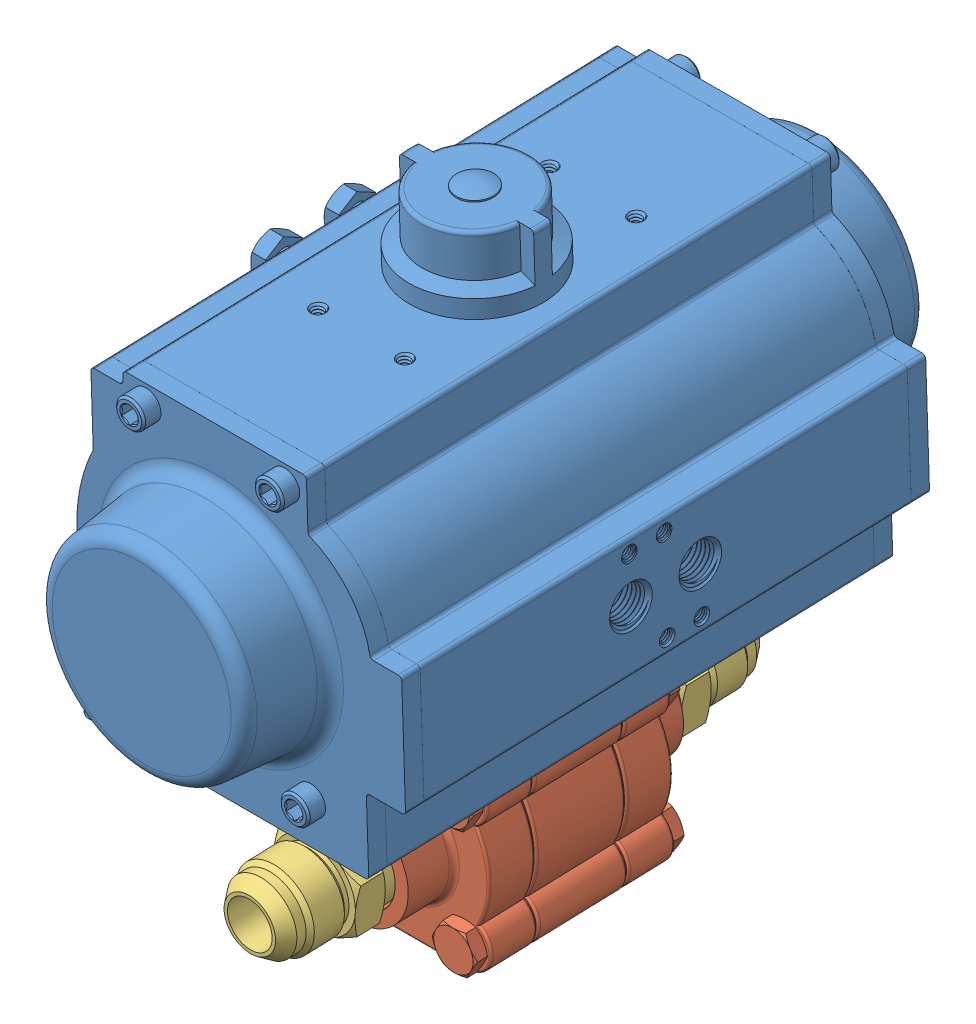
SolidWorks assembly SOV-5, configuration Default. Lengths in mm.
Overall size (123.09 217.36 240.36).
4 component instances, 3 part files, 5 mates.
Components (placement in the parent):
- 49935K880_AIR ACTUATOR FOR BALL-BUTTERFLY VALVE-1: 49935K880_AIR ACTUATOR FOR BALL-BUTTERFLY VALVE [49935K88] at (-134.9516 813.8383 165.2589) x (1 0 0) z (0 -0.032429 0.999474) size (123.09 139.45 235.97)
- FAKE_sharpe_80BV-1: FAKE_sharpe_80BV [3778T941] at (-134.9516 771.6203 163.8891) x (0 0.032429 -0.999474) z (1 0 0) size (95.25 86.36 61.47)
- 5482K126_PRECISION AN 37 DEGREE FLARED TUBE FITTING-1: 5482K126_PRECISION AN 37 DEGREE FLARED TUBE FITTING [5482K126] at (-134.9516 773.5325 104.954) x (0 0.032429 -0.999474) z (0.994125 -0.108183 -0.00351) size (59.61 33 28.57)
- 5482K126_PRECISION AN 37 DEGREE FLARED TUBE FITTING-2: 5482K126_PRECISION AN 37 DEGREE FLARED TUBE FITTING [5482K126] at (-134.9516 769.7081 222.8242) x (0 -0.032429 0.999474) z (-0.994125 0.108183 0.00351) size (59.61 33 28.57)
Mates (geometry in assembly coordinates):
- Concentric302: concentric anti-aligned: circle of 49935K880_AIR ACTUATOR FOR BALL-BUTTERFLY VALVE-1; circle of FAKE_sharpe_80BV-1
- Coincident128: coincident anti-aligned: plane of 49935K880_AIR ACTUATOR FOR BALL-BUTTERFLY VALVE-1 through (-183.9736 810.8987 255.8575) normal (0 -0.999474 -0.032429); plane of FAKE_sharpe_80BV-1 through (-134.9516 813.8383 165.2589) normal (0 0.999474 0.032429)
- Coincident138: coincident aligned: plane of 49935K880_AIR ACTUATOR FOR BALL-BUTTERFLY VALVE-1 through (-134.9516 813.8383 165.2589) normal (1 0 0); plane of FAKE_sharpe_80BV-1 through (-134.9516 771.6203 163.8891) normal (1 0 0)
- Concentric303: concentric aligned: cone of FAKE_sharpe_80BV-1 through (-134.9516 772.7117 130.2518) axis (0 -0.032429 0.999474); cylinder of 5482K126_PRECISION AN 37 DEGREE FLARED TUBE FITTING-1 through (-134.9516 773.2815 112.6906) axis (0 -0.032429 0.999474) radius 10.691
- Distance1: distance = 13.462 mm anti-aligned: plane of 5482K126_PRECISION AN 37 DEGREE FLARED TUBE FITTING-1 through (-134.9516 772.7281 129.7441) normal (0 -0.032429 0.999474); plane of FAKE_sharpe_80BV-1 through (-134.9516 773.1647 116.2891) normal (0 0.032429 -0.999474)
